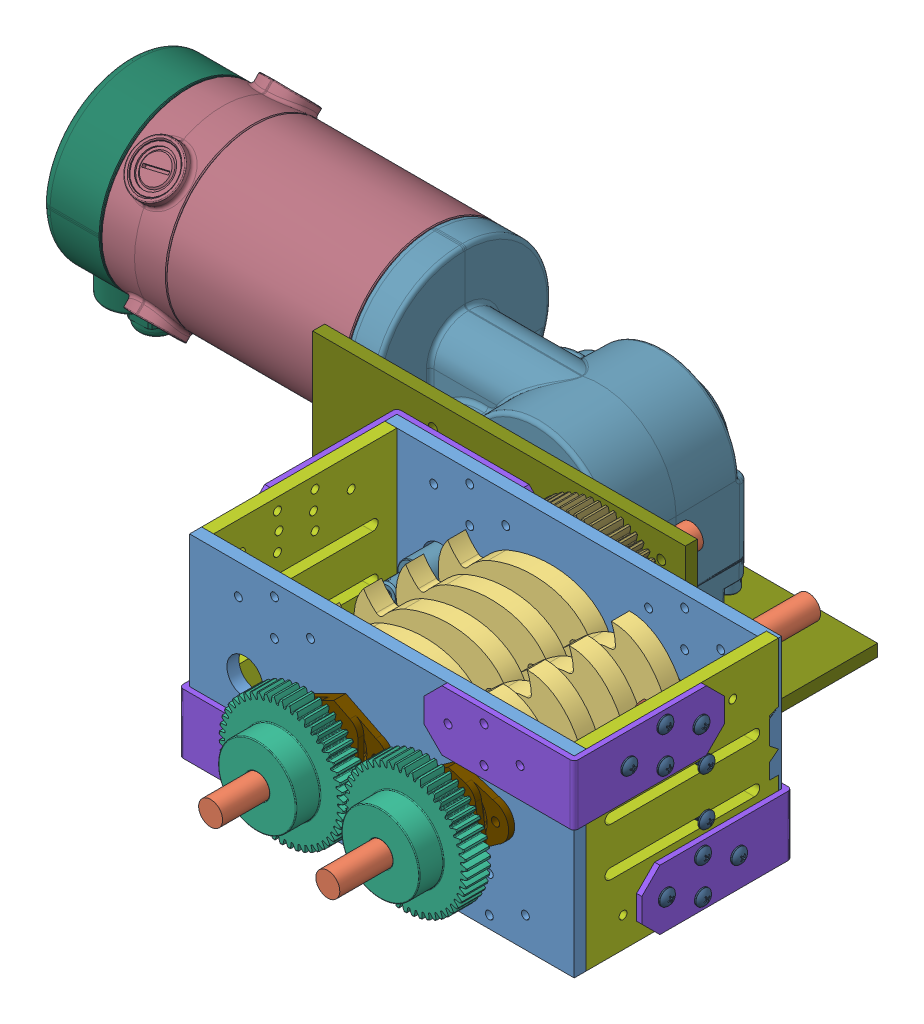
SolidWorks assembly ShredderAssem, configuration Default. Lengths in mm.
Overall size (434.34 143.91 309.56).
63 component instances, 18 part files, 85 mates.
Components (placement in the parent):
- frontWall(forExcessToothOverlap)-3: frontWall(forExcessToothOverlap) [Default] at (-103.9808 46.8763 146.828) size (203.2 101.6 6.35)
- shaftassem-3: shaftassem [Default] at (324.6285 219.1558 351.8159) x (0 0 -1) z (0.309638 0.950854 0) size (254 113.01 112.98)
  - shaft_approx-2: shaft_approx [Default] at (125.6129 231.0581 -203.0005) size (254 12.7 12.7)
  - Blade-9: Blade [Default] at (209.7504 231.0581 -203.0005) x (1 0 0) z (0 0.717916 0.696129) size (9.53 79.05 80.77)
  - grainger-36wy84-1: grainger-36wy84 [Default] at (224.0379 231.0581 -203.0005) x (0 0.857491 -0.514498) z (1 0 0) size (31.74 31.75 9.53)
  - grainger-36wy84-6: grainger-36wy84 [Default] at (246.2629 231.0581 -203.0005) x (0 0.857491 -0.514498) z (1 0 0) size (31.74 31.75 9.53)
  - grainger-36wy84-7: grainger-36wy84 [Default] at (268.4879 231.0581 -203.0005) x (0 0.857491 -0.514498) z (1 0 0) size (31.74 31.75 9.53)
  - grainger-36wy84-8: grainger-36wy84 [Default] at (290.7129 231.0581 -203.0005) x (0 0.857491 -0.514498) z (1 0 0) size (31.74 31.75 9.53)
  - Blade-14: Blade [Default] at (231.9754 231.0581 -203.0005) x (1 0 0) z (0 0.717916 0.696129) size (9.53 79.05 80.77)
  - Blade-15: Blade [Default] at (254.2004 231.0581 -203.0005) x (1 0 0) z (0 0.717916 0.696129) size (9.53 79.05 80.77)
  - Blade-16: Blade [Default] at (276.4254 231.0581 -203.0005) x (1 0 0) z (0 0.717916 0.696129) size (9.53 79.05 80.77)
- shaftassem-4: shaftassem [Default] at (245.389 -55.3081 -154.9974) x (0 0 1) z (0.19891 -0.980018 0) size (254 113.01 112.98)
  - shaft_approx-2: shaft_approx [Default] at (125.6129 231.0581 -203.0005) size (254 12.7 12.7)
  - Blade-9: Blade [Default] at (209.7504 231.0581 -203.0005) x (1 0 0) z (0 0.717916 0.696129) size (9.53 79.05 80.77)
  - grainger-36wy84-1: grainger-36wy84 [Default] at (224.0379 231.0581 -203.0005) x (0 0.857491 -0.514498) z (1 0 0) size (31.74 31.75 9.53)
  - grainger-36wy84-6: grainger-36wy84 [Default] at (246.2629 231.0581 -203.0005) x (0 0.857491 -0.514498) z (1 0 0) size (31.74 31.75 9.53)
  - grainger-36wy84-7: grainger-36wy84 [Default] at (268.4879 231.0581 -203.0005) x (0 0.857491 -0.514498) z (1 0 0) size (31.74 31.75 9.53)
  - grainger-36wy84-8: grainger-36wy84 [Default] at (290.7129 231.0581 -203.0005) x (0 0.857491 -0.514498) z (1 0 0) size (31.74 31.75 9.53)
  - Blade-14: Blade [Default] at (231.9754 231.0581 -203.0005) x (1 0 0) z (0 0.717916 0.696129) size (9.53 79.05 80.77)
  - Blade-15: Blade [Default] at (254.2004 231.0581 -203.0005) x (1 0 0) z (0 0.717916 0.696129) size (9.53 79.05 80.77)
  - Blade-16: Blade [Default] at (276.4254 231.0581 -203.0005) x (1 0 0) z (0 0.717916 0.696129) size (9.53 79.05 80.77)
- frontWall(forExcessToothOverlap)-4: frontWall(forExcessToothOverlap) [Default] at (-103.9808 46.8763 43.6405) size (203.2 101.6 6.35)
- FINGERS-1: FINGERS [Default] at (61.1192 46.8763 87.0308) size (31.75 92.71 6.35)
- 50t-1: 50t [5172T58] at (42.0692 97.6763 185.6952) x (0.720143 0.693826 0) z (0 0 1) size (66.03 66.09 25.43)
- 50t-2: 50t [5172T58] at (-21.4308 97.6763 187.339) x (0.874819 0.484451 0) z (0 0 1) size (66.03 66.09 25.43)
- sideWall-2: sideWall [Default] at (-97.6308 46.8763 151.5905) x (0 0 -1) z (1 0 0) size (101.6 101.6 6.35)
- 17715A67_Galvanized Steel Corner Bracket-3: 17715A67_Galvanized Steel Corner Bracket [17715A67] at (100.6162 132.6013 154.575) x (-1 0 0) z (0 0 -1) size (79.38 31.75 79.38)
- 17715A67_Galvanized Steel Corner Bracket-6: 17715A67_Galvanized Steel Corner Bracket [17715A67] at (-105.3778 132.6013 42.2435) size (79.38 31.75 79.38)
- 17715A67_Galvanized Steel Corner Bracket-11: 17715A67_Galvanized Steel Corner Bracket [17715A67] at (-105.3778 62.7513 154.575) x (1 0 0) z (0 0 -1) size (79.38 31.75 79.38)
- 17715A67_Galvanized Steel Corner Bracket-13: 17715A67_Galvanized Steel Corner Bracket [17715A67] at (100.6162 62.7513 42.2435) x (-1 0 0) z (0 0 1) size (79.38 31.75 79.38)
- sideWall-3: sideWall [Default] at (99.2192 46.8763 146.828) x (0 0 -1) z (1 0 0) size (101.6 101.6 6.35)
- 2780T18_High-Load Ball Bearing-1: 2780T18_High-Load Ball Bearing [2780T18] at (42.0692 97.6763 148.4155) x (0.979601 0.200954 0) z (0 0 1) size (28.57 28.57 9.53)
- 2780T18_High-Load Ball Bearing-2: 2780T18_High-Load Ball Bearing [2780T18] at (-21.4308 97.6763 148.4155) x (0.851068 0.525056 0) z (0 0 1) size (28.57 28.57 9.53)
- 2780T18_High-Load Ball Bearing-4: 2780T18_High-Load Ball Bearing [2780T18] at (42.0692 97.6763 48.403) x (0.988698 -0.14992 0) z (0 0 -1) size (28.57 28.57 9.53)
- 2780T18_High-Load Ball Bearing-6: 2780T18_High-Load Ball Bearing [2780T18] at (-21.4308 97.6763 48.403) x (0.982101 -0.188357 0) z (0 0 -1) size (28.57 28.57 9.53)
- 90272A194_Zinc-Plated Steel Pan Head Phillips Screw-1: 90272A194_Zinc-Plated Steel Pan Head Phillips Screw [90272A194] at (94.3297 110.3763 83.8558) x (0 -0.548612 0.836077) z (1 0 0) size (8.18 8.18 15.67)
- 90272A194_Zinc-Plated Steel Pan Head Phillips Screw-2: 90272A194_Zinc-Plated Steel Pan Head Phillips Screw [90272A194] at (94.3297 84.9763 83.8558) x (0 -0.982696 -0.185224) z (1 0 0) size (8.18 8.18 15.67)
- 90272A194_Zinc-Plated Steel Pan Head Phillips Screw-4: 90272A194_Zinc-Plated Steel Pan Head Phillips Screw [90272A194] at (97.1237 142.1263 108.347) x (0 -0.911548 0.411194) z (1 0 0) size (8.18 8.18 15.67)
- 90272A194_Zinc-Plated Steel Pan Head Phillips Screw-6: 90272A194_Zinc-Plated Steel Pan Head Phillips Screw [90272A194] at (97.1237 123.0763 108.347) x (0 -0.969102 0.246659) z (1 0 0) size (8.18 8.18 15.67)
- 90272A194_Zinc-Plated Steel Pan Head Phillips Screw-8: 90272A194_Zinc-Plated Steel Pan Head Phillips Screw [90272A194] at (97.1237 132.6013 127.397) x (0 -0.997211 0.074629) z (1 0 0) size (8.18 8.18 15.67)
- 90272A194_Zinc-Plated Steel Pan Head Phillips Screw-10: 90272A194_Zinc-Plated Steel Pan Head Phillips Screw [90272A194] at (97.1237 132.6013 89.297) x (0 -0.995021 -0.099669) z (1 0 0) size (8.18 8.18 15.67)
- 90272A194_Zinc-Plated Steel Pan Head Phillips Screw-12: 90272A194_Zinc-Plated Steel Pan Head Phillips Screw [90272A194] at (97.1237 62.7513 107.5215) x (0 -0.962597 -0.270938) z (1 0 0) size (8.18 8.18 15.67)
- 90272A194_Zinc-Plated Steel Pan Head Phillips Screw-14: 90272A194_Zinc-Plated Steel Pan Head Phillips Screw [90272A194] at (97.1237 53.2263 88.4715) x (0 -0.900925 -0.433975) z (1 0 0) size (8.18 8.18 15.67)
- 90272A194_Zinc-Plated Steel Pan Head Phillips Screw-16: 90272A194_Zinc-Plated Steel Pan Head Phillips Screw [90272A194] at (97.1237 72.2763 88.4715) x (0 -0.811879 -0.583826) z (1 0 0) size (8.18 8.18 15.67)
- 90272A194_Zinc-Plated Steel Pan Head Phillips Screw-18: 90272A194_Zinc-Plated Steel Pan Head Phillips Screw [90272A194] at (97.1237 62.7513 69.4215) x (0 -0.698164 -0.715938) z (1 0 0) size (8.18 8.18 15.67)
- 93181A009_Aluminum Hex Nut-1: 93181A009_Aluminum Hex Nut [93181A009] at (91.2817 132.6013 127.397) x (0 0.592983 -0.805215) z (0 -0.805215 -0.592983) size (8.73 3.83 10.08)
- 93181A009_Aluminum Hex Nut-2: 93181A009_Aluminum Hex Nut [93181A009] at (91.2817 142.1263 108.347) x (0 0.713151 -0.701011) z (0 -0.701011 -0.713151) size (8.73 3.83 10.08)
- 93181A009_Aluminum Hex Nut-4: 93181A009_Aluminum Hex Nut [93181A009] at (91.2817 123.0763 108.347) x (0 0.796607 -0.604497) z (0 -0.604497 -0.796607) size (8.73 3.83 10.08)
- 93181A009_Aluminum Hex Nut-6: 93181A009_Aluminum Hex Nut [93181A009] at (91.2817 132.6013 89.297) x (0 0.849485 -0.527612) z (0 -0.527612 -0.849485) size (8.73 3.83 10.08)
- 93181A009_Aluminum Hex Nut-10: 93181A009_Aluminum Hex Nut [93181A009] at (91.2817 62.7513 107.5215) x (0 0.876948 -0.480585) z (0 -0.480585 -0.876948) size (8.73 3.83 10.08)
- 93181A009_Aluminum Hex Nut-12: 93181A009_Aluminum Hex Nut [93181A009] at (91.2817 53.2263 88.4715) x (0 0.881582 -0.472031) z (0 -0.472031 -0.881582) size (8.73 3.83 10.08)
- 93181A009_Aluminum Hex Nut-14: 93181A009_Aluminum Hex Nut [93181A009] at (91.2817 72.2763 88.4715) x (0 0.861621 -0.507552) z (0 -0.507552 -0.861621) size (8.73 3.83 10.08)
- 93181A009_Aluminum Hex Nut-16: 93181A009_Aluminum Hex Nut [93181A009] at (91.2817 62.7513 69.4215) x (0 0.810373 -0.585914) z (0 -0.585914 -0.810373) size (8.73 3.83 10.08)
- 5172T59_Metal Gear - 20 Degree Pressure Angle-1: 5172T59_Metal Gear - 20 Degree Pressure Angle [5172T59] at (-21.4308 97.6763 30.9405) x (0.999681 -0.025249 0) z (0 0 1) size (78.74 78.74 25.43)
- Motor_Assem-1: Motor_Assem [Default] at (11.3936 273.3691 -221) x (-1 0 0) z (0 0 1) size (348.06 128.36 160.99)
  - ElectroCraft-MP26-WR-016V24-020-X-1: ElectroCraft-MP26-WR-016V24-020-X [Default] at (174.2174 154.2298 186.8905) size (290.81 122.01 158.49)
    - ElectroCraft-MP26-WR-016V24-020-X_SA_Motor_MPP26-1: ElectroCraft-MP26-WR-016V24-020-X_SA_Motor_MPP26 [Default] at origin size (129.5 93.09 93.09)
    - ElectroCraft-MP26-WR-016V24-020-X_SA_Gearbox_MP_WR_No_Release-1: ElectroCraft-MP26-WR-016V24-020-X_SA_Gearbox_MP_WR_No_Release [Default] at (-88.053 21.463 0) size (133.21 121.76 158.49)
    - ElectroCraft-MP26-WR-016V24-020-X_SA_MTR_Cover_wo_Encoder-Brake-1: ElectroCraft-MP26-WR-016V24-020-X_SA_MTR_Cover_wo_Encoder-Brake [Default] at (129.5 0 0) size (33.63 117.57 92.76)
  - ShredderMotorMount-1: ShredderMotorMount [Default] at (112.1644 229.6928 186.8905) size (196.85 101.6 101.6)
- 24T-1: 24T [5172T57] at (-74.7708 97.6763 30.1785) x (0.999842 -0.017782 0) z (0 0 1) size (32.91 32.91 23.91)
- Retaining_piece-1: Retaining_piece [Default] at (-21.4308 116.7263 159.528) x (-1 0 0) z (0 0 -1) size (51.83 38.1 6.35)
- Retaining_piece-2: Retaining_piece [Default] at (39.0488 116.4853 159.528) x (-0.987351 -0.158553 0) z (0 0 -1) size (51.83 38.1 6.35)
Mates (geometry in assembly coordinates):
- Concentric1: concentric aligned: circle of frontWall(forExcessToothOverlap)-3; circle of shaftassem-4/shaft_approx-2
- Concentric2: concentric anti-aligned: circle of frontWall(forExcessToothOverlap)-3; circle of shaftassem-3/shaft_approx-2
- Distance1: distance = 6.35 mm anti-aligned: plane of shaftassem-4/grainger-36wy84-8 through (-21.4308 97.6763 140.478) normal (0 0 1); plane of frontWall(forExcessToothOverlap)-3 through (-103.9808 46.8763 146.828) normal (0 0 -1)
- Distance2: distance = 1.5875 mm anti-aligned: plane of shaftassem-4/Blade-16 through (-21.4308 97.6763 130.953) normal (0 0 1); plane of shaftassem-3/Blade-9 through (42.0692 97.6763 132.5405) normal (0 0 -1)
- Concentric3: concentric aligned: circle of shaftassem-4/shaft_approx-2; circle of frontWall(forExcessToothOverlap)-4
- Concentric4: concentric anti-aligned: circle of shaftassem-3/shaft_approx-2; circle of frontWall(forExcessToothOverlap)-4
- Distance3: distance = 6.35 mm anti-aligned: plane of shaftassem-3/grainger-36wy84-8 through (42.0692 97.6763 56.3405) normal (0 0 -1); plane of frontWall(forExcessToothOverlap)-4 through (-103.9808 46.8763 49.9905) normal (0 0 1)
- Concentric7: concentric aligned: cylinder of shaftassem-3/shaft_approx-2 through (42.0692 97.6763 -27.797) axis (0 0 1) radius 6.35; cylinder of 50t-1 through (42.0692 97.6763 198.3952) axis (0 0 1) radius 6.35
- Concentric9: concentric anti-aligned: cylinder of shaftassem-4/shaft_approx-2 through (-21.4308 97.6763 224.6155) axis (0 0 -1) radius 6.35; cylinder of 50t-2 through (-21.4308 97.6763 200.039) axis (0 0 1) radius 6.35
- Coincident11: coincident anti-aligned: plane of frontWall(forExcessToothOverlap)-4 through (-103.9808 46.8763 49.9905) normal (0 0 1); plane of sideWall-2 through (-97.6308 148.4763 49.9905) normal (0 0 -1)
- Coincident12: coincident aligned: plane of frontWall(forExcessToothOverlap)-3 through (-103.9808 148.4763 153.178) normal (0 1 0); plane of sideWall-2 through (-97.6308 148.4763 151.5905) normal (0 1 0)
- Coincident13: coincident aligned: plane of frontWall(forExcessToothOverlap)-3 through (-103.9808 46.8763 153.178) normal (-1 0 0); plane of sideWall-2 through (-103.9808 148.4763 151.5905) normal (-1 0 0)
- Coincident21: coincident anti-aligned: plane of frontWall(forExcessToothOverlap)-3 through (-103.9808 46.8763 153.178) normal (0 0 1); plane of 17715A67_Galvanized Steel Corner Bracket-3 through (99.2192 148.4763 153.178) normal (0 0 -1)
- Coincident23: coincident aligned: plane of frontWall(forExcessToothOverlap)-4 through (-103.9808 148.4763 49.9905) normal (0 1 0); plane of 17715A67_Galvanized Steel Corner Bracket-6 through (-105.3778 148.4763 42.2435) normal (0 1 0)
- Coincident26: coincident anti-aligned: plane of frontWall(forExcessToothOverlap)-4 through (-103.9808 46.8763 43.6405) normal (0 0 -1); plane of 17715A67_Galvanized Steel Corner Bracket-6 through (-103.9808 148.4763 43.6405) normal (0 0 1)
- Coincident27: coincident anti-aligned: plane of sideWall-2 through (-103.9808 148.4763 151.5905) normal (-1 0 0); plane of 17715A67_Galvanized Steel Corner Bracket-6 through (-103.9808 148.4763 120.2215) normal (1 0 0)
- Coincident36: coincident aligned: plane of frontWall(forExcessToothOverlap)-3 through (-103.9808 46.8763 153.178) normal (0 -1 0); plane of 17715A67_Galvanized Steel Corner Bracket-11 through (-105.3778 46.8763 154.575) normal (0 -1 0)
- Coincident37: coincident anti-aligned: plane of frontWall(forExcessToothOverlap)-3 through (-103.9808 46.8763 153.178) normal (0 0 1); plane of 17715A67_Galvanized Steel Corner Bracket-11 through (-103.9808 46.8763 153.178) normal (0 0 -1)
- Coincident38: coincident anti-aligned: plane of sideWall-2 through (-103.9808 148.4763 151.5905) normal (-1 0 0); plane of 17715A67_Galvanized Steel Corner Bracket-11 through (-103.9808 46.8763 76.597) normal (1 0 0)
- Coincident39: coincident aligned: plane of frontWall(forExcessToothOverlap)-4 through (-103.9808 46.8763 49.9905) normal (0 -1 0); plane of 17715A67_Galvanized Steel Corner Bracket-13 through (100.6162 46.8763 42.2435) normal (0 -1 0)
- Coincident40: coincident anti-aligned: plane of frontWall(forExcessToothOverlap)-4 through (-103.9808 46.8763 43.6405) normal (0 0 -1); plane of 17715A67_Galvanized Steel Corner Bracket-13 through (99.2192 46.8763 43.6405) normal (0 0 1)
- Coincident41: coincident anti-aligned: plane of frontWall(forExcessToothOverlap)-3 through (-103.9808 46.8763 146.828) normal (0 0 -1); plane of sideWall-3 through (99.2192 148.4763 146.828) normal (0 0 1)
- Coincident44: coincident aligned: plane of frontWall(forExcessToothOverlap)-3 through (-103.9808 46.8763 153.178) normal (0 -1 0); plane of sideWall-3 through (99.2192 46.8763 146.828) normal (0 -1 0)
- Coincident45: coincident aligned: plane of frontWall(forExcessToothOverlap)-3 through (99.2192 46.8763 153.178) normal (1 0 0); plane of sideWall-3 through (99.2192 148.4763 146.828) normal (1 0 0)
- Coincident46: coincident anti-aligned: plane of 17715A67_Galvanized Steel Corner Bracket-3 through (99.2192 148.4763 76.597) normal (-1 0 0); plane of sideWall-3 through (99.2192 148.4763 146.828) normal (1 0 0)
- Coincident47: coincident aligned: plane of frontWall(forExcessToothOverlap)-3 through (-103.9808 148.4763 153.178) normal (0 1 0); plane of 17715A67_Galvanized Steel Corner Bracket-3 through (100.6162 148.4763 154.575) normal (0 1 0)
- Coincident48: coincident anti-aligned: plane of 17715A67_Galvanized Steel Corner Bracket-13 through (99.2192 46.8763 120.2215) normal (-1 0 0); plane of sideWall-3 through (99.2192 148.4763 146.828) normal (1 0 0)
- Concentric10: concentric aligned: cylinder of frontWall(forExcessToothOverlap)-3 through (42.0692 97.6763 106.4168) axis (0 0 1) radius 14.2875; cylinder of 2780T18_High-Load Ball Bearing-1 through (42.0692 97.6763 153.178) axis (0 0 1) radius 14.2875
- Coincident50: coincident aligned: plane of frontWall(forExcessToothOverlap)-3 through (-103.9808 46.8763 153.178) normal (0 0 1); plane of 2780T18_High-Load Ball Bearing-1 through (39.2938 111.2058 153.178) normal (0 0 1)
- Concentric11: concentric aligned: cylinder of frontWall(forExcessToothOverlap)-3 through (-21.4308 97.6763 106.4168) axis (0 0 1) radius 14.2875; cylinder of 2780T18_High-Load Ball Bearing-2 through (-21.4308 97.6763 153.178) axis (0 0 1) radius 14.2875
- Coincident51: coincident aligned: plane of frontWall(forExcessToothOverlap)-3 through (-103.9808 46.8763 153.178) normal (0 0 1); plane of 2780T18_High-Load Ball Bearing-2 through (-28.6824 109.4306 153.178) normal (0 0 1)
- Concentric12: concentric anti-aligned: cylinder of frontWall(forExcessToothOverlap)-4 through (42.0692 97.6763 3.2293) axis (0 0 1) radius 14.2875; cylinder of 2780T18_High-Load Ball Bearing-4 through (42.0692 97.6763 43.6405) axis (0 0 -1) radius 14.2875
- Coincident52: coincident aligned: plane of frontWall(forExcessToothOverlap)-4 through (-103.9808 46.8763 43.6405) normal (0 0 -1); plane of 2780T18_High-Load Ball Bearing-4 through (39.9986 84.0211 43.6405) normal (0 0 -1)
- Concentric13: concentric anti-aligned: cylinder of frontWall(forExcessToothOverlap)-4 through (-21.4308 97.6763 3.2293) axis (0 0 1) radius 14.2875; cylinder of 2780T18_High-Load Ball Bearing-6 through (-21.4308 97.6763 43.6405) axis (0 0 -1) radius 14.2875
- Coincident53: coincident aligned: plane of frontWall(forExcessToothOverlap)-4 through (-103.9808 46.8763 43.6405) normal (0 0 -1); plane of 2780T18_High-Load Ball Bearing-6 through (-24.0322 84.1123 43.6405) normal (0 0 -1)
- Coincident54: coincident aligned: plane of FINGERS-1 through (61.1192 46.8763 87.0308) normal (0 -1 0); plane of sideWall-3 through (99.2192 46.8763 146.828) normal (0 -1 0)
- Coincident55: coincident anti-aligned: plane of FINGERS-1 through (92.8692 148.4763 87.0308) normal (1 0 0); plane of sideWall-3 through (92.8692 148.4763 146.828) normal (-1 0 0)
- Concentric141: concentric aligned: cylinder of FINGERS-1 through (92.8692 110.3763 83.8558) axis (1 0 0) radius 1.7272; cylinder of 90272A194_Zinc-Plated Steel Pan Head Phillips Screw-1 through (102.1402 110.3763 83.8558) axis (1 0 0) radius 2.0828
- Coincident57: coincident anti-aligned: plane of sideWall-3 through (99.2192 148.4763 146.828) normal (1 0 0); plane of 90272A194_Zinc-Plated Steel Pan Head Phillips Screw-1 through (99.2192 108.2473 87.1004) normal (-1 0 0)
- Concentric15: concentric aligned: cylinder of FINGERS-1 through (92.8692 84.9763 83.8558) axis (1 0 0) radius 1.7272; cylinder of 90272A194_Zinc-Plated Steel Pan Head Phillips Screw-2 through (102.1402 84.9763 83.8558) axis (1 0 0) radius 2.0828
- Coincident58: coincident anti-aligned: plane of sideWall-3 through (99.2192 148.4763 146.828) normal (1 0 0); plane of 90272A194_Zinc-Plated Steel Pan Head Phillips Screw-2 through (99.2192 81.1627 83.137) normal (-1 0 0)
- Concentric16: concentric anti-aligned: cylinder of 17715A67_Galvanized Steel Corner Bracket-3 through (102.0142 142.1263 108.347) axis (-1 0 0) radius 2.0828; cylinder of 90272A194_Zinc-Plated Steel Pan Head Phillips Screw-4 through (104.9342 142.1263 108.347) axis (1 0 0) radius 2.0828
- Coincident59: coincident anti-aligned: plane of 17715A67_Galvanized Steel Corner Bracket-3 through (102.0132 148.4763 155.972) normal (1 0 0); plane of 90272A194_Zinc-Plated Steel Pan Head Phillips Screw-4 through (102.0132 138.5888 109.9427) normal (-1 0 0)
- Concentric17: concentric anti-aligned: cylinder of 17715A67_Galvanized Steel Corner Bracket-3 through (102.0142 123.0763 108.347) axis (-1 0 0) radius 2.0828; cylinder of 90272A194_Zinc-Plated Steel Pan Head Phillips Screw-6 through (104.9342 123.0763 108.347) axis (1 0 0) radius 2.0828
- Coincident60: coincident anti-aligned: plane of 17715A67_Galvanized Steel Corner Bracket-3 through (102.0132 148.4763 155.972) normal (1 0 0); plane of 90272A194_Zinc-Plated Steel Pan Head Phillips Screw-6 through (102.0132 119.3154 109.3042) normal (-1 0 0)
- Concentric18: concentric anti-aligned: cylinder of 17715A67_Galvanized Steel Corner Bracket-3 through (102.0142 132.6013 127.397) axis (-1 0 0) radius 2.0828; cylinder of 90272A194_Zinc-Plated Steel Pan Head Phillips Screw-8 through (104.9342 132.6013 127.397) axis (1 0 0) radius 2.0828
- Coincident61: coincident anti-aligned: plane of 17715A67_Galvanized Steel Corner Bracket-3 through (102.0132 148.4763 155.972) normal (1 0 0); plane of 90272A194_Zinc-Plated Steel Pan Head Phillips Screw-8 through (102.0132 128.7314 127.6866) normal (-1 0 0)
- Concentric19: concentric anti-aligned: cylinder of 17715A67_Galvanized Steel Corner Bracket-3 through (102.0142 132.6013 89.297) axis (-1 0 0) radius 2.0828; cylinder of 90272A194_Zinc-Plated Steel Pan Head Phillips Screw-10 through (104.9342 132.6013 89.297) axis (1 0 0) radius 2.0828
- Coincident62: coincident anti-aligned: plane of 17715A67_Galvanized Steel Corner Bracket-3 through (102.0132 148.4763 155.972) normal (1 0 0); plane of 90272A194_Zinc-Plated Steel Pan Head Phillips Screw-10 through (102.0132 128.7399 88.9102) normal (-1 0 0)
- Concentric20: concentric anti-aligned: cylinder of 17715A67_Galvanized Steel Corner Bracket-13 through (102.0142 62.7513 107.5215) axis (-1 0 0) radius 2.0828; cylinder of 90272A194_Zinc-Plated Steel Pan Head Phillips Screw-12 through (104.9342 62.7513 107.5215) axis (1 0 0) radius 2.0828
- Coincident63: coincident anti-aligned: plane of 17715A67_Galvanized Steel Corner Bracket-13 through (102.0132 46.8763 40.8465) normal (1 0 0); plane of 90272A194_Zinc-Plated Steel Pan Head Phillips Screw-12 through (102.0132 59.0157 106.47) normal (-1 0 0)
- Concentric21: concentric anti-aligned: cylinder of 17715A67_Galvanized Steel Corner Bracket-13 through (102.0142 53.2263 88.4715) axis (-1 0 0) radius 2.0828; cylinder of 90272A194_Zinc-Plated Steel Pan Head Phillips Screw-14 through (104.9342 53.2263 88.4715) axis (1 0 0) radius 2.0828
- Coincident64: coincident anti-aligned: plane of 17715A67_Galvanized Steel Corner Bracket-13 through (102.0132 46.8763 40.8465) normal (1 0 0); plane of 90272A194_Zinc-Plated Steel Pan Head Phillips Screw-14 through (102.0132 49.73 86.7873) normal (-1 0 0)
- Concentric22: concentric anti-aligned: cylinder of 17715A67_Galvanized Steel Corner Bracket-13 through (102.0142 72.2763 88.4715) axis (-1 0 0) radius 2.0828; cylinder of 90272A194_Zinc-Plated Steel Pan Head Phillips Screw-16 through (104.9342 72.2763 88.4715) axis (1 0 0) radius 2.0828
- Coincident65: coincident anti-aligned: plane of 17715A67_Galvanized Steel Corner Bracket-13 through (102.0132 46.8763 40.8465) normal (1 0 0); plane of 90272A194_Zinc-Plated Steel Pan Head Phillips Screw-16 through (102.0132 69.1256 86.2058) normal (-1 0 0)
- Concentric23: concentric anti-aligned: cylinder of 17715A67_Galvanized Steel Corner Bracket-13 through (102.0142 62.7513 69.4215) axis (-1 0 0) radius 2.0828; cylinder of 90272A194_Zinc-Plated Steel Pan Head Phillips Screw-18 through (104.9342 62.7513 69.4215) axis (1 0 0) radius 2.0828
- Coincident66: coincident anti-aligned: plane of 17715A67_Galvanized Steel Corner Bracket-13 through (102.0132 46.8763 40.8465) normal (1 0 0); plane of 90272A194_Zinc-Plated Steel Pan Head Phillips Screw-18 through (102.0132 60.0419 66.6431) normal (-1 0 0)
- Concentric24: concentric anti-aligned: circle of sideWall-3; circle of 93181A009_Aluminum Hex Nut-1
- Coincident68: coincident anti-aligned: plane of sideWall-3 through (92.8692 148.4763 146.828) normal (-1 0 0); plane of 93181A009_Aluminum Hex Nut-1 through (92.8692 132.0421 132.4069) normal (1 0 0)
- Concentric25: concentric anti-aligned: circle of sideWall-3; circle of 93181A009_Aluminum Hex Nut-2
- Coincident69: coincident anti-aligned: plane of sideWall-3 through (92.8692 148.4763 146.828) normal (-1 0 0); plane of 93181A009_Aluminum Hex Nut-2 through (92.8692 140.7798 113.2048) normal (1 0 0)
- Concentric26: concentric anti-aligned: circle of sideWall-3; circle of 93181A009_Aluminum Hex Nut-4
- Coincident70: coincident anti-aligned: plane of sideWall-3 through (92.8692 148.4763 146.828) normal (-1 0 0); plane of 93181A009_Aluminum Hex Nut-4 through (92.8692 121.1222 112.9938) normal (1 0 0)
- Concentric27: concentric anti-aligned: circle of sideWall-3; circle of 93181A009_Aluminum Hex Nut-6
- Coincident71: coincident anti-aligned: plane of sideWall-3 through (92.8692 148.4763 146.828) normal (-1 0 0); plane of 93181A009_Aluminum Hex Nut-6 through (92.8692 130.2226 93.7415) normal (1 0 0)
- Concentric28: concentric anti-aligned: circle of sideWall-3; circle of 93181A009_Aluminum Hex Nut-10
- Coincident72: coincident anti-aligned: plane of sideWall-3 through (92.8692 148.4763 146.828) normal (-1 0 0); plane of 93181A009_Aluminum Hex Nut-10 through (92.8692 60.1342 111.8299) normal (1 0 0)
- Concentric29: concentric anti-aligned: circle of sideWall-3; circle of 93181A009_Aluminum Hex Nut-12
- Coincident73: coincident anti-aligned: plane of sideWall-3 through (92.8692 148.4763 146.828) normal (-1 0 0); plane of 93181A009_Aluminum Hex Nut-12 through (92.8692 50.5674 92.7542) normal (1 0 0)
- Concentric30: concentric anti-aligned: circle of sideWall-3; circle of 93181A009_Aluminum Hex Nut-14
- Coincident74: coincident anti-aligned: plane of sideWall-3 through (92.8692 148.4763 146.828) normal (-1 0 0); plane of 93181A009_Aluminum Hex Nut-14 through (92.8692 69.7941 92.859) normal (1 0 0)
- Concentric31: concentric anti-aligned: circle of sideWall-3; circle of 93181A009_Aluminum Hex Nut-16
- Coincident75: coincident anti-aligned: plane of sideWall-3 through (92.8692 148.4763 146.828) normal (-1 0 0); plane of 93181A009_Aluminum Hex Nut-16 through (92.8692 60.6903 74.0219) normal (1 0 0)
- Concentric143: concentric anti-aligned: cylinder of shaftassem-4/shaft_approx-2 through (-21.4308 97.6763 224.6155) axis (0 0 -1) radius 6.35; cylinder of 5172T59_Metal Gear - 20 Degree Pressure Angle-1 through (-21.4308 97.6763 43.6405) axis (0 0 1) radius 6.35
- Concentric144: concentric aligned: cylinder of frontWall(forExcessToothOverlap)-4 through (-74.7708 97.6763 3.2293) axis (0 0 1) radius 9.525; cylinder of Motor_Assem-1/ElectroCraft-MP26-WR-016V24-020-X-1/ElectroCraft-MP26-WR-016V24-020-X_SA_Gearbox_MP_WR_No_Release-1 through (-74.7708 97.6763 40.9299) axis (0 0 1) radius 8.4798
- Parallel1: parallel aligned: plane of frontWall(forExcessToothOverlap)-4 through (-103.9808 148.4763 49.9905) normal (0 1 0); plane of Motor_Assem-1/ShredderMotorMount-1 through (-100.7708 138.9263 -34.1095) normal (0 1 0)
- Coincident77: coincident anti-aligned: plane of frontWall(forExcessToothOverlap)-4 through (-103.9808 46.8763 43.6405) normal (0 0 -1); plane of 5172T59_Metal Gear - 20 Degree Pressure Angle-1 through (-21.4308 97.6763 43.6405) normal (0 0 1)
- Coincident78: coincident anti-aligned: plane of 5172T59_Metal Gear - 20 Degree Pressure Angle-1 through (-21.4308 97.6763 18.2405) normal (0 0 -1); plane of Motor_Assem-1/ShredderMotorMount-1 through (-173.872 37.3263 18.2405) normal (0 0 1)
- Parallel2: parallel aligned: cylinder of shaftassem-4/shaft_approx-2 through (-21.4308 97.6763 224.6155) axis (0 0 -1) radius 6.35; cylinder of Motor_Assem-1/ShredderMotorMount-1 through (-21.332 97.6763 18.2405) axis (0 0 -1) radius 14.2875
- Concentric146: concentric aligned: cylinder of Motor_Assem-1/ElectroCraft-MP26-WR-016V24-020-X-1/ElectroCraft-MP26-WR-016V24-020-X_SA_Gearbox_MP_WR_No_Release-1 through (-74.7708 97.6763 40.9299) axis (0 0 1) radius 8.4798; cylinder of 24T-1 through (-74.7708 97.6763 42.1165) axis (0 0 1) radius 6.35
- Coincident80: coincident anti-aligned: plane of Motor_Assem-1/ShredderMotorMount-1 through (-173.872 37.3263 18.2405) normal (0 0 1); plane of 24T-1 through (-74.7708 97.6763 18.2405) normal (0 0 -1)
- Concentric147: concentric anti-aligned: cylinder of shaftassem-4/shaft_approx-2 through (-21.4308 97.6763 224.6155) axis (0 0 -1) radius 6.35; cylinder of Retaining_piece-1 through (-21.4308 97.6763 153.178) axis (0 0 1) radius 8.255
- Coincident81: coincident anti-aligned: plane of frontWall(forExcessToothOverlap)-3 through (-103.9808 46.8763 153.178) normal (0 0 1); plane of Retaining_piece-1 through (-37.3058 97.6763 153.178) normal (0 0 -1)
- Coincident82: coincident anti-aligned: plane of frontWall(forExcessToothOverlap)-3 through (-103.9808 46.8763 153.178) normal (0 0 1); plane of Retaining_piece-2 through (26.395 95.1593 153.178) normal (0 0 -1)
- Concentric149: concentric aligned: cylinder of shaftassem-3/shaft_approx-2 through (42.0692 97.6763 -27.797) axis (0 0 1) radius 6.35; cylinder of Retaining_piece-2 through (42.0692 97.6763 153.178) axis (0 0 1) radius 8.255
